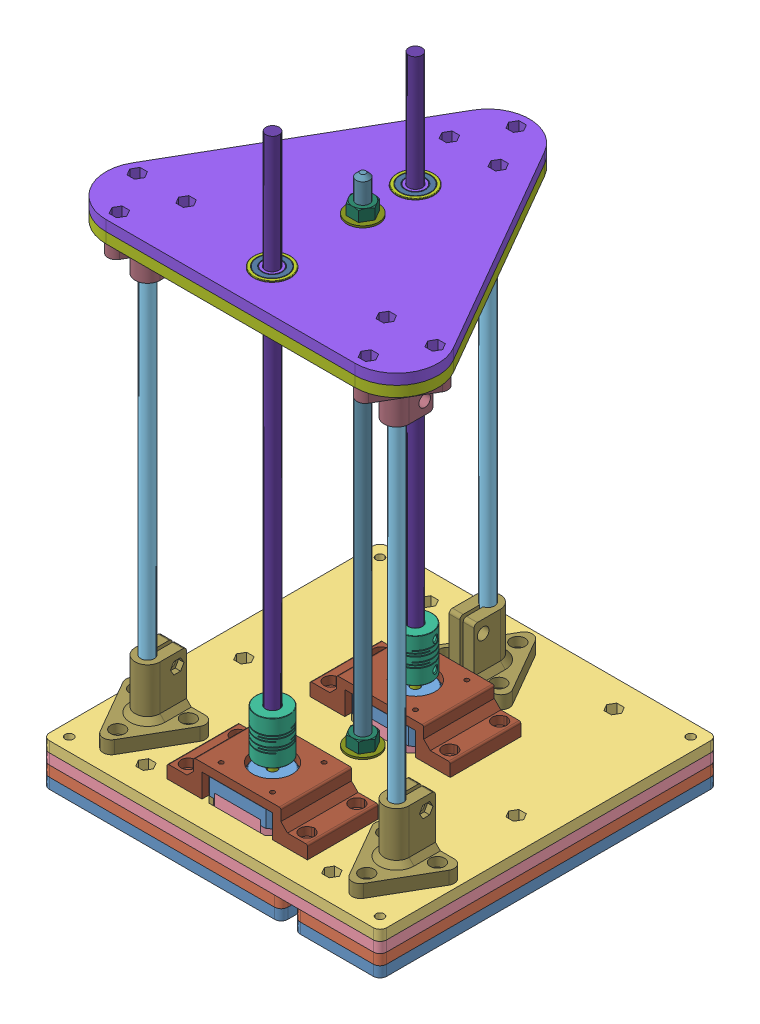
SolidWorks assembly 02_00_Assy_z_axis_V1, configuration Défaut. Lengths in mm.
Overall size (203.2 380.91 203.2).
110 component instances, 54 part files, 67 mates.
Components (placement in the parent):
- 02_01_Assy_base_z_axis_V1-1: 02_01_Assy_base_z_axis_V1 [Défaut] at (-233.6469 0 294.9138) size (203.2 25.4 203.2)
  - 02_03_plaque_fond_base-1: 02_03_plaque_fond_base [Défaut] at (80.101 0 119.7934) size (203.2 6.35 203.2)
  - 02_05_deuxieme_niveau_base-1: 02_05_deuxieme_niveau_base [Défaut] at (80.101 6.35 119.7934) x (-1 0 0) z (0 0 -1) size (203.2 6.35 203.2)
  - 02_06_troixieme_niveau_base-1: 02_06_troixieme_niveau_base [Défaut] at (80.101 19.05 119.7934) x (-1 0 0) z (0 0 -1) size (203.2 6.35 203.2)
  - 02_012_deuxieme_v2_niveau_base-1: 02_012_deuxieme_v2_niveau_base [Défaut] at (80.101 12.7 119.7934) x (-1 0 0) z (0 0 -1) size (203.2 6.35 203.2)
- Stainless_Steel_Rod_8_290-1: Stainless_Steel_Rod_8_290 [1274T471] at (-228.5459 151.35 479.7071) x (0.927753 0 -0.373195) z (0 -1 0) size (8 8 290)
- Stainless_Steel_Rod_8_290-2: Stainless_Steel_Rod_8_290 [1274T471] at (-78.5444 151.35 479.7063) x (-0.988682 0 -0.150024) z (0 -1 0) size (8 8 290)
- Stainless_Steel_Rod_8_290-3: Stainless_Steel_Rod_8_290 [1274T471] at (-153.5459 151.35 349.7071) x (-0.878649 0 -0.477467) z (0 1 0) size (8 8 290)
- NEMA17_Coupler-1: NEMA17_Coupler [Default] at (-153.3959 48.5 479.5571) x (-0.967472 0 -0.252977) z (0.252977 0 -0.967472) size (26.77 26 23.11)
- 02_09_support_trois_rods_haut-1: 02_09_support_trois_rods_haut [Défaut] at (-153.5451 290 414.7071) x (-1 0 0.000011) z (-0.000011 0 -1) size (200 6.35 180)
- 02_10_support_haut-1: 02_10_support_haut [Défaut] at (-153.5451 296.35 414.7071) x (-1 0 0.000011) z (-0.000011 0 -1) size (200 6.35 180)
- 608-2RS Skate Board Ball Bearing.step-2: 608-2RS Skate Board Ball Bearing.step [Default] at (-153.5444 299.85 479.7071) x (0 -1 0) z (0 0 1) size (7 22 22)
  - Ball 001.step-1: Ball 001.step [Default] at origin size (4 4 4)
  - Ball 002.step-1: Ball 002.step [Default] x (1 0 0) z (0 0.781831 0.62349) size (4 4 4)
  - Ball 003.step-1: Ball 003.step [Default] x (1 0 0) z (0 0.974928 -0.222521) size (4 4 4)
  - Ball 004.step-1: Ball 004.step [Default] x (1 0 0) z (0 0.433884 -0.900969) size (4 4 4)
  - Ball 005.step-1: Ball 005.step [Default] x (1 0 0) z (0 -0.433884 -0.900969) size (4 4 4)
  - Ball 006.step-1: Ball 006.step [Default] x (1 0 0) z (0 -0.974928 -0.222521) size (4 4 4)
  - Ball 007.step-1: Ball 007.step [Default] x (1 0 0) z (0 -0.781831 0.62349) size (4 4 4)
  - Cage 001.step-1: Cage 001.step [Default] x (1 0 0) z (0 1 0) size (2.12 17 16.8)
  - Cage 002.step-1: Cage 002.step [Default] x (-1 0 0) z (0 0 -1) size (2.12 16.8 17)
  - Rivet 001.step-1: Rivet 001.step [Default] x (1 0 0) z (0 -0.433884 0.900969) size (0.42 0.6 0.6)
  - Rivet 002.step-1: Rivet 002.step [Default] x (1 0 0) z (0 -0.781831 0.62349) size (0.42 0.6 0.6)
  - Rivet 003.step-1: Rivet 003.step [Default] x (1 0 0) z (0 -0.974928 -0.222521) size (0.42 0.6 0.6)
  - Rivet 004.step-1: Rivet 004.step [Default] x (1 0 0) z (0 -0.433884 -0.900969) size (0.42 0.6 0.6)
  - Rivet 005.step-1: Rivet 005.step [Default] x (1 0 0) z (0 0.433884 -0.900969) size (0.42 0.6 0.6)
  - Rivet 006.step-1: Rivet 006.step [Default] x (1 0 0) z (0 0.974928 -0.222521) size (0.42 0.6 0.6)
  - Rivet 007.step-1: Rivet 007.step [Default] x (1 0 0) z (0 0.781831 0.62349) size (0.42 0.6 0.6)
  - Outer Ring001.step-1: Outer Ring001.step [Default] at origin size (7 22 22)
  - Inner Ring001.step-1: Inner Ring001.step [Default] at origin size (7 12 12)
  - Seal 001.step-1: Seal 001.step [Default] at origin size (0.6 19 19)
  - Seal 002.step-1: Seal 002.step [Default] x (-1 0 0) z (0 0 -1) size (0.6 19 19)
- 02_11_support_moteur-1: 02_11_support_moteur [Défaut] at (-153.3959 39.5 479.5571) size (84.5 19.1 42.5)
- 02_13_support_rodes_8mm_base-1: 02_13_support_rodes_8mm_base [Défaut] at (-78.5444 25.4 479.7063) x (-1 0 0) z (0 0 -1) size (47.68 37.8 42.63)
- 02_13_support_rodes_8mm_base-2: 02_13_support_rodes_8mm_base [Défaut] at (-228.5459 25.4 479.7071) x (-1 0 0) z (0 0 -1) size (47.68 37.8 42.63)
- 02_13_support_rodes_8mm_base-3: 02_13_support_rodes_8mm_base [Défaut] at (-153.5459 25.4 349.7071) size (47.68 37.8 42.63)
- 02_14_support_rodes_8mm_haut-1: 02_14_support_rodes_8mm_haut [Défaut] at (-78.5444 290 479.7063) x (1 0 -0.000011) z (-0.000011 0 -1) size (42.68 27.8 38.3)
- 02_14_support_rodes_8mm_haut-2: 02_14_support_rodes_8mm_haut [Défaut] at (-228.5459 290 479.7071) x (1 0 -0.000011) z (-0.000011 0 -1) size (42.68 27.8 38.3)
- 02_14_support_rodes_8mm_haut-3: 02_14_support_rodes_8mm_haut [Défaut] at (-153.5459 290 349.7071) x (-1 0 0.000011) z (0.000011 0 1) size (42.68 27.8 38.3)
- Lead Screw_M12-1: Lead Screw_M12 [97048A742] at (-153.5459 162.5 425.0321) x (-0.414721 0 0.909949) z (0 -1 0) size (7.9 7.9 325)
- 95462A510_Medium-Strength Steel Hex Nut-2: 95462A510_Medium-Strength Steel Hex Nut [95462A510] at (-153.5459 307.1656 425.0321) x (0.86602 0 -0.50001) z (0 1 0) size (12.7 14.66 6.75)
- 516_washer-1: 516_washer [90107A030] at (-153.5459 302.7 425.0321) size (19.05 1.09 19.05)
- 516_washer-2: 516_washer [90107A030] at (-153.5459 25.4 425.0321) size (19.05 1.09 19.05)
- T8_lead_screw_300mm-1: T8_lead_screw_300mm [1274T471] at (-153.3959 223.9115 479.5571) x (0.654232 0 0.756294) z (0 1 0) size (8 8 300)
- 02_11_support_moteur-2: 02_11_support_moteur [Défaut] at (-153.3959 39.5 393.5571) size (84.5 19.1 42.5)
- 95462A510_Medium-Strength Steel Hex Nut-4: 95462A510_Medium-Strength Steel Hex Nut [95462A510] at (-153.5459 29.8656 425.0321) x (0.866025 0 -0.5) z (0 1 0) size (12.7 14.66 6.75)
- 608-2RS Skate Board Ball Bearing.step-3: 608-2RS Skate Board Ball Bearing.step [Default] at (-153.3959 299.85 393.5571) x (0 -1 0) z (0.672808 0 0.739817) size (7 22 22)
  - Ball 001.step-1: Ball 001.step [Default] at origin size (4 4 4)
  - Ball 002.step-1: Ball 002.step [Default] x (1 0 0) z (0 0.781831 0.62349) size (4 4 4)
  - Ball 003.step-1: Ball 003.step [Default] x (1 0 0) z (0 0.974928 -0.222521) size (4 4 4)
  - Ball 004.step-1: Ball 004.step [Default] x (1 0 0) z (0 0.433884 -0.900969) size (4 4 4)
  - Ball 005.step-1: Ball 005.step [Default] x (1 0 0) z (0 -0.433884 -0.900969) size (4 4 4)
  - Ball 006.step-1: Ball 006.step [Default] x (1 0 0) z (0 -0.974928 -0.222521) size (4 4 4)
  - Ball 007.step-1: Ball 007.step [Default] x (1 0 0) z (0 -0.781831 0.62349) size (4 4 4)
  - Cage 001.step-1: Cage 001.step [Default] x (1 0 0) z (0 1 0) size (2.12 17 16.8)
  - Cage 002.step-1: Cage 002.step [Default] x (-1 0 0) z (0 0 -1) size (2.12 16.8 17)
  - Rivet 001.step-1: Rivet 001.step [Default] x (1 0 0) z (0 -0.433884 0.900969) size (0.42 0.6 0.6)
  - Rivet 002.step-1: Rivet 002.step [Default] x (1 0 0) z (0 -0.781831 0.62349) size (0.42 0.6 0.6)
  - Rivet 003.step-1: Rivet 003.step [Default] x (1 0 0) z (0 -0.974928 -0.222521) size (0.42 0.6 0.6)
  - Rivet 004.step-1: Rivet 004.step [Default] x (1 0 0) z (0 -0.433884 -0.900969) size (0.42 0.6 0.6)
  - Rivet 005.step-1: Rivet 005.step [Default] x (1 0 0) z (0 0.433884 -0.900969) size (0.42 0.6 0.6)
  - Rivet 006.step-1: Rivet 006.step [Default] x (1 0 0) z (0 0.974928 -0.222521) size (0.42 0.6 0.6)
  - Rivet 007.step-1: Rivet 007.step [Default] x (1 0 0) z (0 0.781831 0.62349) size (0.42 0.6 0.6)
  - Outer Ring001.step-1: Outer Ring001.step [Default] at origin size (7 22 22)
  - Inner Ring001.step-1: Inner Ring001.step [Default] at origin size (7 12 12)
  - Seal 001.step-1: Seal 001.step [Default] at origin size (0.6 19 19)
  - Seal 002.step-1: Seal 002.step [Default] x (-1 0 0) z (0 0 -1) size (0.6 19 19)
- NEMA17_Coupler-2: NEMA17_Coupler [Default] at (-153.3959 48.5 393.5571) x (-0.262561 0 -0.964915) z (0.964915 0 -0.262561) size (26.77 26 23.11)
- T8_lead_screw_300mm-2: T8_lead_screw_300mm [1274T471] at (-153.3959 222.3941 393.5571) x (0.983512 0 0.18084) z (0 -1 0) size (8 8 300)
- 95462A510_Medium-Strength Steel Hex Nut-5: 95462A510_Medium-Strength Steel Hex Nut [95462A510] at (-153.5459 3.3734 425.0321) x (0.866025 0 -0.5) z (0 -1 0) size (12.7 14.66 6.75)
- NEMA17 x 33.step-1: NEMA17 x 33.step [Défaut] at (-153.3959 39.5 393.5571) x (0 0 1) z (1 0 0) size (42 70.5 60)
  - Copper-2of4.step-1: Copper-2of4.step [Défaut] at (0 28 0) x (0 1 0) z (0 0 1) size (2.77 3.05 24)
  - Frontplate.step-1: Frontplate.step [Défaut] at (0 10.5 0) size (42 12.5 42)
  - Backplate.step-1: Backplate.step [Défaut] at (0 33 0) size (42 10.5 42)
  - Connenctor.step-1: Connenctor.step [Défaut] at (0 24.5 22) size (7 7 7)
  - Housing.step-1: Housing.step [Défaut] at (0 7.5 0) size (42 32 42)
  - Bearing dummy.step-1: Bearing dummy.step [Défaut] at (0 4 0) size (22 7 22)
  - Bearing dummy 01.step-1: Bearing dummy 01.step [Défaut] at (0 28 0) size (22 7 22)
  - Core.step-1: Core.step [Défaut] at origin size (30 70.5 30)
  - M3x25-Screw.step-1: M3x25-Screw.step [Défaut] at (15.5 30.6 15.5) x (1 0 0) z (0 1 0) size (5.5 5.5 27)
  - M3x25-Screw004.step-1: M3x25-Screw004.step [Défaut] at (-15.5 30.6 15.5) x (1 0 0) z (0 1 0) size (5.5 5.5 27)
  - M3x25-Screw005.step-1: M3x25-Screw005.step [Défaut] at (-15.5 30.6 -15.5) x (1 0 0) z (0 1 0) size (5.5 5.5 27)
  - M3x25-Screw006.step-1: M3x25-Screw006.step [Défaut] at (15.5 30.6 -15.5) x (1 0 0) z (0 1 0) size (5.5 5.5 27)
  - Cable-1of4.step-1: Cable-1of4.step [Défaut] at (0 28 0) size (3.44 3.69 21)
  - Copper-1of4.step-1: Copper-1of4.step [Défaut] at (0 28 0) size (2.77 3.05 24)
  - Cable-2of4.step-1: Cable-2of4.step [Défaut] at (0 28 0) x (0 1 0) z (0 0 1) size (3.44 3.69 21)
  - Copper-4of4.step-1: Copper-4of4.step [Défaut] at (0 28 0) x (0 -1 0) z (0 0 1) size (2.77 3.05 24)
  - Cable-3of4.step-1: Cable-3of4.step [Défaut] at (0 28 0) x (-1 0 0) z (0 0 1) size (3.44 3.69 21)
  - Copper-3of4.step-1: Copper-3of4.step [Défaut] at (0 28 0) x (-1 0 0) z (0 0 1) size (2.77 3.05 24)
  - Cable-4of4.step-1: Cable-4of4.step [Défaut] at (0 28 0) x (0 -1 0) z (0 0 1) size (3.44 3.69 21)
- NEMA17 x 33.step-2: NEMA17 x 33.step [Défaut] at (-153.3959 39.5 479.5571) x (0 0 1) z (1 0 0) size (42 70.5 60)
  - Copper-2of4.step-1: Copper-2of4.step [Défaut] at (0 28 0) x (0 1 0) z (0 0 1) size (2.77 3.05 24)
  - Frontplate.step-1: Frontplate.step [Défaut] at (0 10.5 0) size (42 12.5 42)
  - Backplate.step-1: Backplate.step [Défaut] at (0 33 0) size (42 10.5 42)
  - Connenctor.step-1: Connenctor.step [Défaut] at (0 24.5 22) size (7 7 7)
  - Housing.step-1: Housing.step [Défaut] at (0 7.5 0) size (42 32 42)
  - Bearing dummy.step-1: Bearing dummy.step [Défaut] at (0 4 0) size (22 7 22)
  - Bearing dummy 01.step-1: Bearing dummy 01.step [Défaut] at (0 28 0) size (22 7 22)
  - Core.step-1: Core.step [Défaut] at origin size (30 70.5 30)
  - M3x25-Screw.step-1: M3x25-Screw.step [Défaut] at (15.5 30.6 15.5) x (1 0 0) z (0 1 0) size (5.5 5.5 27)
  - M3x25-Screw004.step-1: M3x25-Screw004.step [Défaut] at (-15.5 30.6 15.5) x (1 0 0) z (0 1 0) size (5.5 5.5 27)
  - M3x25-Screw005.step-1: M3x25-Screw005.step [Défaut] at (-15.5 30.6 -15.5) x (1 0 0) z (0 1 0) size (5.5 5.5 27)
  - M3x25-Screw006.step-1: M3x25-Screw006.step [Défaut] at (15.5 30.6 -15.5) x (1 0 0) z (0 1 0) size (5.5 5.5 27)
  - Cable-1of4.step-1: Cable-1of4.step [Défaut] at (0 28 0) size (3.44 3.69 21)
  - Copper-1of4.step-1: Copper-1of4.step [Défaut] at (0 28 0) size (2.77 3.05 24)
  - Cable-2of4.step-1: Cable-2of4.step [Défaut] at (0 28 0) x (0 1 0) z (0 0 1) size (3.44 3.69 21)
  - Copper-4of4.step-1: Copper-4of4.step [Défaut] at (0 28 0) x (0 -1 0) z (0 0 1) size (2.77 3.05 24)
  - Cable-3of4.step-1: Cable-3of4.step [Défaut] at (0 28 0) x (-1 0 0) z (0 0 1) size (3.44 3.69 21)
  - Copper-3of4.step-1: Copper-3of4.step [Défaut] at (0 28 0) x (-1 0 0) z (0 0 1) size (2.77 3.05 24)
  - Cable-4of4.step-1: Cable-4of4.step [Défaut] at (0 28 0) x (0 -1 0) z (0 0 1) size (3.44 3.69 21)
Mates (geometry in assembly coordinates):
- Coïncidente1: coincident anti-aligned: plane of 02_01_Assy_base_z_axis_V1-1/02_03_plaque_fond_base-1 through (-153.5459 0 414.7071) normal (0 -1 0)
- Coïncidente4: coincident anti-aligned: plane of 02_01_Assy_base_z_axis_V1-1/02_03_plaque_fond_base-1 through (-153.5459 6.35 414.7071) normal (0 1 0); plane of Stainless_Steel_Rod_8_290-1 through (-228.5459 6.35 479.7071) normal (0 -1 0)
- Coïncidente5: coincident anti-aligned: plane of 02_01_Assy_base_z_axis_V1-1/02_03_plaque_fond_base-1 through (-153.5459 6.35 414.7071) normal (0 1 0); plane of Stainless_Steel_Rod_8_290-2 through (-78.5444 6.35 479.7063) normal (0 -1 0)
- Coïncidente6: coincident anti-aligned: plane of 02_01_Assy_base_z_axis_V1-1/02_03_plaque_fond_base-1 through (-153.5459 6.35 414.7071) normal (0 1 0); plane of Stainless_Steel_Rod_8_290-3 through (-153.5459 6.35 349.7071) normal (0 -1 0)
- Coïncidente29: coincident aligned: plane of Stainless_Steel_Rod_8_290-1 through (-228.5459 296.35 479.7071) normal (0 1 0); plane of 02_09_support_trois_rods_haut-1 through (-78.5444 296.35 479.7063) normal (0 1 0)
- Coaxiale20: concentric aligned: cylinder of Stainless_Steel_Rod_8_290-3 through (-153.5459 296.35 349.7071) axis (0 -1 0) radius 4; cylinder of 02_09_support_trois_rods_haut-1 through (-153.5459 296.35 349.7071) axis (0 -1 0) radius 3.925
- Coaxiale21: concentric anti-aligned: cylinder of Stainless_Steel_Rod_8_290-2 through (-78.5444 6.35 479.7063) axis (0 1 0) radius 4; cylinder of 02_09_support_trois_rods_haut-1 through (-78.5444 296.35 479.7063) axis (0 -1 0) radius 3.925
- Coïncidente30: coincident anti-aligned: plane of 02_09_support_trois_rods_haut-1 through (-78.5444 296.35 479.7063) normal (0 1 0); plane of 02_10_support_haut-1 through (-78.5444 296.35 479.7063) normal (0 -1 0)
- Coaxiale22: concentric aligned: cylinder of 02_09_support_trois_rods_haut-1 through (-153.5444 296.35 479.7071) axis (0 -1 0) radius 5.7; cylinder of 02_10_support_haut-1 through (-153.5444 302.7 479.7071) axis (0 -1 0) radius 11
- Coïncidente31: coincident aligned: plane of 02_09_support_trois_rods_haut-1 through (-56.8899 296.35 467.213) normal (0.86618 0 -0.499732); plane of 02_10_support_haut-1 through (-56.8899 302.7 467.213) normal (0.86618 0 -0.499732)
- Coaxiale26: concentric aligned: cylinder of Stainless_Steel_Rod_8_290-2 through (-78.5444 6.35 479.7063) axis (0 1 0) radius 4; cylinder of 02_13_support_rodes_8mm_base-1 through (-78.5444 25.4 479.7063) axis (0 1 0) radius 4.075
- Coïncidente36: coincident anti-aligned: plane of 02_01_Assy_base_z_axis_V1-1/02_06_troixieme_niveau_base-1 through (-153.5459 25.4 414.7071) normal (0 1 0); plane of 02_13_support_rodes_8mm_base-1 through (-78.5444 25.4 479.7063) normal (0 -1 0)
- Coaxiale27: concentric anti-aligned: cylinder of Stainless_Steel_Rod_8_290-3 through (-153.5459 296.35 349.7071) axis (0 -1 0) radius 4; cylinder of 02_13_support_rodes_8mm_base-3 through (-153.5459 25.4 349.7071) axis (0 1 0) radius 4.075
- Coïncidente38: coincident anti-aligned: plane of 02_01_Assy_base_z_axis_V1-1/02_06_troixieme_niveau_base-1 through (-153.5459 25.4 414.7071) normal (0 1 0); plane of 02_13_support_rodes_8mm_base-3 through (-153.5459 25.4 349.7071) normal (0 -1 0)
- Parallèle3: parallel anti-aligned: plane of 02_01_Assy_base_z_axis_V1-1/02_06_troixieme_niveau_base-1 through (-51.9459 25.4 516.3071) normal (0 0 1); plane of 02_13_support_rodes_8mm_base-1 through (-51.0444 33.2 463.8292) normal (0 0 -1)
- Coïncidente41: coincident anti-aligned: plane of 02_01_Assy_base_z_axis_V1-1/02_06_troixieme_niveau_base-1 through (-153.5459 25.4 414.7071) normal (0 1 0); plane of 02_13_support_rodes_8mm_base-2 through (-228.5459 25.4 479.7071) normal (0 -1 0)
- Coaxiale28: concentric aligned: cylinder of Stainless_Steel_Rod_8_290-1 through (-228.5459 6.35 479.7071) axis (0 1 0) radius 4; cylinder of 02_13_support_rodes_8mm_base-2 through (-228.5459 25.4 479.7071) axis (0 1 0) radius 4.075
- Parallèle4: parallel anti-aligned: plane of 02_01_Assy_base_z_axis_V1-1/02_06_troixieme_niveau_base-1 through (-51.9459 25.4 516.3071) normal (0 0 1); plane of 02_13_support_rodes_8mm_base-2 through (-201.0459 33.2 463.83) normal (0 0 -1)
- Coïncidente46: coincident anti-aligned: plane of 02_09_support_trois_rods_haut-1 through (-78.5444 290 479.7063) normal (0 -1 0); plane of 02_14_support_rodes_8mm_haut-2 through (-228.5459 290 479.7071) normal (0 1 0)
- Coaxiale30: concentric anti-aligned: cylinder of Stainless_Steel_Rod_8_290-1 through (-228.5459 6.35 479.7071) axis (0 1 0) radius 4; cylinder of 02_14_support_rodes_8mm_haut-2 through (-228.5459 290 479.7071) axis (0 -1 0) radius 4.075
- Parallèle5: parallel anti-aligned: plane of 02_09_support_trois_rods_haut-1 through (-78.5441 296.35 504.7063) normal (0.000011 0 1); plane of 02_14_support_rodes_8mm_haut-2 through (-253.546 282.2 465.2737) normal (-0.000011 0 -1)
- Coïncidente48: coincident anti-aligned: plane of 02_09_support_trois_rods_haut-1 through (-78.5444 290 479.7063) normal (0 -1 0); plane of 02_14_support_rodes_8mm_haut-1 through (-78.5444 290 479.7063) normal (0 1 0)
- Coaxiale31: concentric anti-aligned: cylinder of 02_14_support_rodes_8mm_haut-1 through (-78.5444 290 479.7063) axis (0 -1 0) radius 4.075; cylinder of Stainless_Steel_Rod_8_290-2 through (-78.5444 6.35 479.7063) axis (0 1 0) radius 4
- Parallèle7: parallel anti-aligned: plane of 02_09_support_trois_rods_haut-1 through (-78.5441 296.35 504.7063) normal (0.000011 0 1); plane of 02_14_support_rodes_8mm_haut-1 through (-103.5446 282.2 465.2728) normal (-0.000011 0 -1)
- Coïncidente51: coincident anti-aligned: plane of 02_09_support_trois_rods_haut-1 through (-78.5444 290 479.7063) normal (0 -1 0); plane of 02_14_support_rodes_8mm_haut-3 through (-153.5459 290 349.7071) normal (0 1 0)
- Coaxiale32: concentric aligned: cylinder of Stainless_Steel_Rod_8_290-3 through (-153.5459 296.35 349.7071) axis (0 -1 0) radius 4; cylinder of 02_14_support_rodes_8mm_haut-3 through (-153.5459 290 349.7071) axis (0 -1 0) radius 4.075
- Coaxiale34: concentric anti-aligned: cylinder of 02_10_support_haut-1 through (-153.5459 296.35 425.0321) axis (0 1 0) radius 4; cylinder of Lead Screw_M12-1 through (-153.5459 0 425.0321) axis (0 -1 0) radius 3.95
- Coïncidente52: coincident aligned: plane of 02_01_Assy_base_z_axis_V1-1/02_03_plaque_fond_base-1 through (-153.5459 0 414.7071) normal (0 -1 0); plane of Lead Screw_M12-1 through (-157.1402 0 423.394) normal (0 -1 0)
- Coaxiale38: concentric anti-aligned: cylinder of 02_01_Assy_base_z_axis_V1-1/02_06_troixieme_niveau_base-1 through (-153.5459 19.05 349.7071) axis (0 1 0) radius 3.925; cylinder of Stainless_Steel_Rod_8_290-3 through (-153.5459 296.35 349.7071) axis (0 -1 0) radius 4
- Parallèle13: parallel anti-aligned: plane of 02_01_Assy_base_z_axis_V1-1/02_03_plaque_fond_base-1 through (-255.1459 6.35 313.1071) normal (0 0 -1); plane of 02_13_support_rodes_8mm_base-3 through (-181.0459 33.2 365.5843) normal (0 0 1)
- Parallèle14: parallel aligned: plane of 02_09_support_trois_rods_haut-1 through (-78.5441 296.35 504.7063) normal (0.000011 0 1); plane of 02_14_support_rodes_8mm_haut-3 through (-128.5457 282.2 364.1406) normal (0.000011 0 1)
- Coaxiale43: concentric aligned: cylinder of 02_01_Assy_base_z_axis_V1-1/02_06_troixieme_niveau_base-1 through (-228.5459 19.05 479.7071) axis (0 1 0) radius 3.925; cylinder of Stainless_Steel_Rod_8_290-1 through (-228.5459 6.35 479.7071) axis (0 1 0) radius 4
- Parallèle15: parallel anti-aligned: plane of 02_01_Assy_base_z_axis_V1-1/02_06_troixieme_niveau_base-1 through (-51.9459 25.4 516.3071) normal (0 0 1); plane of 02_13_support_rodes_8mm_base-2 through (-201.0459 33.2 463.83) normal (0 0 -1)
- Coaxiale48: concentric aligned: cylinder of Lead Screw_M12-1 through (-153.5459 0 425.0321) axis (0 -1 0) radius 3.95; cylinder of 95462A510_Medium-Strength Steel Hex Nut-2 through (-153.5459 310.5391 425.0321) axis (0 -1 0) radius 3.9688
- Coaxiale49: concentric anti-aligned: cylinder of Lead Screw_M12-1 through (-153.5459 0 425.0321) axis (0 -1 0) radius 3.95; cylinder of 516_washer-1 through (-153.5459 302.7 425.0321) axis (0 1 0) radius 4.3688
- Coïncidente69: coincident anti-aligned: plane of 02_10_support_haut-1 through (-78.5444 302.7 479.7063) normal (0 1 0); plane of 516_washer-1 through (-153.5459 302.7 425.0321) normal (0 -1 0)
- Coïncidente70: coincident anti-aligned: plane of 95462A510_Medium-Strength Steel Hex Nut-2 through (-160.8782 303.7922 425.0322) normal (0 -1 0); plane of 516_washer-1 through (-153.5459 303.7922 425.0321) normal (0 1 0)
- Parallèle19: parallel aligned: plane of 02_10_support_haut-1 through (-78.5441 302.7 504.7063) normal (0.000011 0 1); plane of 95462A510_Medium-Strength Steel Hex Nut-2 through (-157.212 310.5391 431.3822) normal (0.000011 0 1)
- Coïncidente72: coincident anti-aligned: plane of 02_01_Assy_base_z_axis_V1-1/02_06_troixieme_niveau_base-1 through (-153.5459 25.4 414.7071) normal (0 1 0); plane of 516_washer-2 through (-153.5459 25.4 425.0321) normal (0 -1 0)
- Coaxiale53: concentric aligned: cylinder of NEMA17_Coupler-1 through (-153.3959 48.5 479.5571) axis (0 -1 0) radius 4.025; cylinder of T8_lead_screw_300mm-1 through (-153.3959 373.9115 479.5571) axis (0 -1 0) radius 4
- Coaxiale58: concentric aligned: cylinder of 02_01_Assy_base_z_axis_V1-1/02_06_troixieme_niveau_base-1 through (-153.5459 19.05 425.0321) axis (0 1 0) radius 4; cylinder of 516_washer-2 through (-153.5459 25.4 425.0321) axis (0 1 0) radius 4.3688
- Coïncidente84: coincident aligned: plane of 02_11_support_moteur-1 through (-179.6459 39.5 479.5571) normal (-1 0 0); plane of 02_11_support_moteur-2 through (-179.6459 39.5 393.5571) normal (-1 0 0)
- Coaxiale61: concentric anti-aligned: cylinder of Lead Screw_M12-1 through (-153.5459 0 425.0321) axis (0 -1 0) radius 3.95; circle of 95462A510_Medium-Strength Steel Hex Nut-4
- Coïncidente89: coincident anti-aligned: plane of 516_washer-2 through (-153.5459 26.4922 425.0321) normal (0 1 0); plane of 95462A510_Medium-Strength Steel Hex Nut-4 through (-160.8782 26.4922 425.0321) normal (0 -1 0)
- Parallèle25: parallel aligned: plane of 02_01_Assy_base_z_axis_V1-1/02_06_troixieme_niveau_base-1 through (-51.9459 25.4 516.3071) normal (0 0 1); plane of 95462A510_Medium-Strength Steel Hex Nut-4 through (-157.2121 33.2391 431.3821) normal (0 0 1)
- Coaxiale64: concentric anti-aligned: cylinder of NEMA17_Coupler-2 through (-153.3959 48.5 393.5571) axis (0 -1 0) radius 4.025; cylinder of T8_lead_screw_300mm-2 through (-153.3959 72.3941 393.5571) axis (0 1 0) radius 4
- Coaxiale65: concentric anti-aligned: cylinder of Lead Screw_M12-1 through (-153.5459 0 425.0321) axis (0 -1 0) radius 3.95; cylinder of 95462A510_Medium-Strength Steel Hex Nut-5 through (-153.5459 0 425.0321) axis (0 1 0) radius 3.9688
- Coaxiale66: concentric anti-aligned: cylinder of 02_01_Assy_base_z_axis_V1-1/02_012_deuxieme_v2_niveau_base-1 through (-153.5459 12.7 425.0321) axis (0 1 0) radius 4; cylinder of Lead Screw_M12-1 through (-153.5459 0 425.0321) axis (0 -1 0) radius 3.95
- Parallèle26: parallel aligned: plane of 02_01_Assy_base_z_axis_V1-1/02_03_plaque_fond_base-1 through (-157.1976 0 418.7071) normal (0.866025 0 0.5); plane of 95462A510_Medium-Strength Steel Hex Nut-5 through (-146.2135 0 425.0321) normal (0.866025 0 0.5)
- Coïncidente95: coincident aligned: plane of 02_01_Assy_base_z_axis_V1-1/02_03_plaque_fond_base-1 through (-153.5459 0 414.7071) normal (0 -1 0); plane of 95462A510_Medium-Strength Steel Hex Nut-5 through (-157.2121 0 431.3821) normal (0 -1 0)
- Coïncidente97: coincident aligned: plane of 02_01_Assy_base_z_axis_V1-1/02_03_plaque_fond_base-1 through (-153.5459 0 414.7071) normal (0 -1 0); plane of NEMA17 x 33.step-2/Housing.step-1 through (-153.3959 0 479.5571) normal (0 -1 0)
- Coïncidente98: coincident aligned: plane of 02_01_Assy_base_z_axis_V1-1/02_03_plaque_fond_base-1 through (-153.5459 0 414.7071) normal (0 -1 0); plane of NEMA17 x 33.step-1/Housing.step-1 through (-153.3959 0 393.5571) normal (0 -1 0)
- Coïncidente99: coincident anti-aligned: plane of 02_01_Assy_base_z_axis_V1-1/02_03_plaque_fond_base-1 through (-132.3959 0 462.7291) normal (-1 0 0); plane of NEMA17 x 33.step-2/Housing.step-1 through (-132.3959 32 465.718) normal (1 0 0)
- Coïncidente100: coincident anti-aligned: plane of 02_01_Assy_base_z_axis_V1-1/02_06_troixieme_niveau_base-1 through (-136.5678 19.05 458.5571) normal (0 0 1); plane of NEMA17 x 33.step-2/Frontplate.step-1 through (-136.4253 29 458.5571) normal (0 0 -1)
- Coïncidente101: coincident anti-aligned: plane of 02_01_Assy_base_z_axis_V1-1/02_06_troixieme_niveau_base-1 through (-132.3959 19.05 376.7291) normal (-1 0 0); plane of NEMA17 x 33.step-1/Frontplate.step-1 through (-132.3959 29 410.5277) normal (1 0 0)
- Coïncidente102: coincident anti-aligned: plane of 02_01_Assy_base_z_axis_V1-1/02_06_troixieme_niveau_base-1 through (-170.5239 19.05 372.5571) normal (0 0 1); plane of NEMA17 x 33.step-1/Frontplate.step-1 through (-136.4253 29 372.5571) normal (0 0 -1)
- Coïncidente103: coincident anti-aligned: plane of NEMA17_Coupler-1 through (-156.0758 48.5 478.8564) normal (0 -1 0); plane of NEMA17 x 33.step-2/Core.step-1 through (-151.1459 48.5 479.5571) normal (0 1 0)
- Coaxiale69: concentric aligned: circle of NEMA17_Coupler-1; cylinder of NEMA17 x 33.step-2/Core.step-1 through (-153.3959 63.2 479.5571) axis (0 -1 0) radius 2.5
- Coïncidente104: coincident anti-aligned: plane of NEMA17_Coupler-2 through (-154.1232 48.5 390.8843) normal (0 -1 0); plane of NEMA17 x 33.step-1/Core.step-1 through (-151.1459 48.5 393.5571) normal (0 1 0)
- Coaxiale70: concentric aligned: circle of NEMA17_Coupler-2; cylinder of NEMA17 x 33.step-1/Core.step-1 through (-153.3959 63.2 393.5571) axis (0 -1 0) radius 2.5
- Coaxiale73: concentric anti-aligned: cylinder of 02_11_support_moteur-1 through (-168.8959 39.5 495.0571) axis (0 1 0) radius 1.325; cylinder of NEMA17 x 33.step-2/Frontplate.step-1 through (-168.8959 29 495.0571) axis (0 -1 0) radius 1.23
- Coaxiale74: concentric anti-aligned: cylinder of 02_11_support_moteur-1 through (-137.8959 39.5 464.0571) axis (0 1 0) radius 1.325; cylinder of NEMA17 x 33.step-2/Frontplate.step-1 through (-137.8959 29 464.0571) axis (0 -1 0) radius 1.23
- Coïncidente106: coincident anti-aligned: plane of 02_11_support_moteur-1 through (-153.3959 39.5 479.5571) normal (0 -1 0); plane of NEMA17 x 33.step-2/Frontplate.step-1 through (-153.3959 39.5 479.5571) normal (0 1 0)
- Coaxiale75: concentric anti-aligned: cylinder of 02_11_support_moteur-2 through (-137.8959 39.5 409.0571) axis (0 1 0) radius 1.325; cylinder of NEMA17 x 33.step-1/Frontplate.step-1 through (-137.8959 29 409.0571) axis (0 -1 0) radius 1.23
- Coïncidente107: coincident anti-aligned: plane of 02_11_support_moteur-2 through (-153.3959 39.5 393.5571) normal (0 -1 0); plane of NEMA17 x 33.step-1/Frontplate.step-1 through (-153.3959 39.5 393.5571) normal (0 1 0)
- Coaxiale76: concentric aligned: cylinder of 608-2RS Skate Board Ball Bearing.step-3/Inner Ring001.step-1 through (-153.3959 296.35 393.5571) axis (0 1 0) radius 4; cylinder of T8_lead_screw_300mm-2 through (-153.3959 72.3941 393.5571) axis (0 1 0) radius 4
- Coïncidente108: coincident anti-aligned: plane of 02_09_support_trois_rods_haut-1 through (-78.5444 296.35 479.7063) normal (0 1 0); plane of 608-2RS Skate Board Ball Bearing.step-3/Outer Ring001.step-1 through (-153.3959 296.35 393.5571) normal (0 -1 0)
